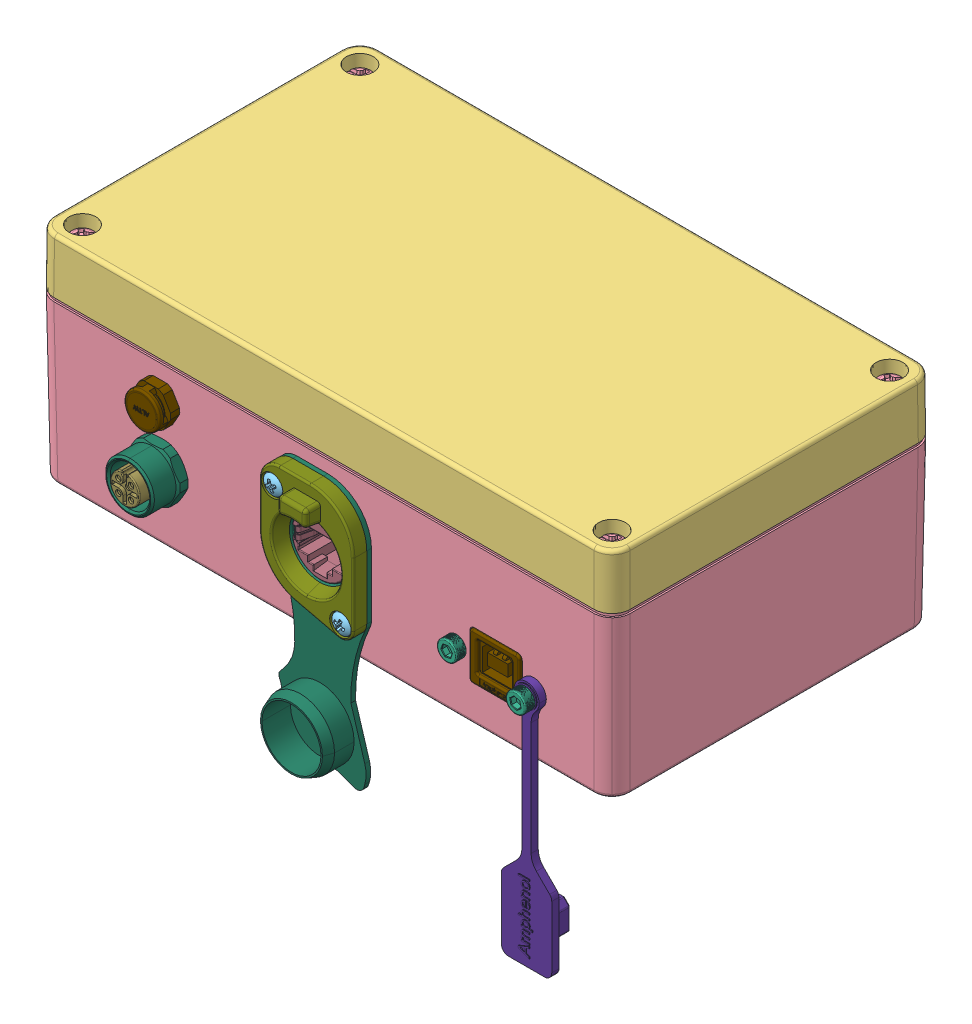
SolidWorks assembly Fleet-Monitor_V1.0, configuration Standard. Lengths in mm.
Overall size (180.3 108.03 100.3).
533 component instances, 174 part files, 48 mates.
Components (placement in the parent):
- Free-Models-1: Free-Models [Standard] x (1 0 0) z (0 1 0) size (180.29 89.97 48.51)
  - 1554J-Body-1: 1554J-Body [Standard] at (-67.276 32.873 34.5) x (1 0 0) z (0 -1 0) size (159.97 48.51 89.97)
    - 1554J.stp-1: 1554J.stp [Standard] at origin size (159.97 48.51 89.97)
      - IN100 (insert M3-0.5X5.75mm BRASS).stp-1: IN100 (insert M3-0.5X5.75mm BRASS).stp [Standard] at (128.026 -41.715 61.8734) size (4.83 5.72 4.83)
      - IN100 (insert M3-0.5X5.75mm BRASS).stp-2: IN100 (insert M3-0.5X5.75mm BRASS).stp [Standard] at (128.026 -41.715 3.8734) size (4.83 5.72 4.83)
      - IN100 (insert M3-0.5X5.75mm BRASS).stp-3: IN100 (insert M3-0.5X5.75mm BRASS).stp [Standard] at (6.526 -41.715 61.8734) size (4.83 5.72 4.83)
      - IN100 (insert M3-0.5X5.75mm BRASS).stp-4: IN100 (insert M3-0.5X5.75mm BRASS).stp [Standard] at (6.526 -41.715 3.8734) size (4.83 5.72 4.83)
      - IN-M4 (insert M4-0.7X5.75mm SS).stp-1: IN-M4 (insert M4-0.7X5.75mm SS).stp [Standard] at (-6.224 -6.35 -5.6266) size (6.35 6.35 6.35)
      - IN-M4 (insert M4-0.7X5.75mm SS).stp-2: IN-M4 (insert M4-0.7X5.75mm SS).stp [Standard] at (-6.224 -6.35 71.3734) size (6.35 6.35 6.35)
      - IN-M4 (insert M4-0.7X5.75mm SS).stp-3: IN-M4 (insert M4-0.7X5.75mm SS).stp [Standard] at (140.776 -6.35 71.3734) size (6.35 6.35 6.35)
      - IN-M4 (insert M4-0.7X5.75mm SS).stp-4: IN-M4 (insert M4-0.7X5.75mm SS).stp [Standard] at (140.776 -6.35 -5.6266) size (6.35 6.35 6.35)
      - 1554J-K GASKET.stp-1: 1554J-K GASKET.stp [Standard] at (-3.2352 3.5 71.7099) x (1 0 0) z (0 -1 0) size (157.48 87.47 1.5)
      - 1554J Box.stp-1: 1554J Box.stp [Standard] x (1 0 0) z (0 1 0) size (159.97 89.97 47.51)
  - M3 x 0.5mm Thread 6mm LONG SOCKET HEAD CAP SCREW-1: M3 x 0.5mm Thread 6mm LONG SOCKET HEAD CAP SCREW [Standard] at (0 29 -6) x (1 0 0) z (0 0 -1) size (5.5 5.5 9)
  - M3 x 0.5mm Thread 6mm LONG SOCKET HEAD CAP SCREW-2: M3 x 0.5mm Thread 6mm LONG SOCKET HEAD CAP SCREW [Standard] at (-60.75 -29 -6) x (1 0 0) z (0 0 -1) size (5.5 5.5 9)
  - M3 x 0.5mm Thread 6mm LONG SOCKET HEAD CAP SCREW-3: M3 x 0.5mm Thread 6mm LONG SOCKET HEAD CAP SCREW [Standard] at (-60.75 29 -6) x (1 0 0) z (0 0 -1) size (5.5 5.5 9)
  - M3 x 0.5mm Thread 6mm LONG SOCKET HEAD CAP SCREW-4: M3 x 0.5mm Thread 6mm LONG SOCKET HEAD CAP SCREW [Standard] at (60.75 29 -6) x (1 0 0) z (0 0 -1) size (5.5 5.5 9)
  - M3 x 0.5mm Thread 6mm LONG SOCKET HEAD CAP SCREW-5: M3 x 0.5mm Thread 6mm LONG SOCKET HEAD CAP SCREW [Standard] at (60.75 -29 -6) x (1 0 0) z (0 0 -1) size (5.5 5.5 9)
  - c-1-967402-1-d2-3d_Receptacle-1: c-1-967402-1-d2-3d_Receptacle [Standard] at (-56.0339 -0.0004 14.3035) x (0.002273 0.984808 -0.173633) z (0.999914 0 0.01309) size (36.5 35.21 44)
- C1-1: C1 [Standard] x (1 0 0) z (0 1 0) size (0.81 1.61 0.81)
  - C1-subassembly-1-1: C1-subassembly-1 [Standard] at (63.6949 12.2289 0) x (0 -1 0) z (0 0 1) size (1.61 0.81 0.81)
    - User Library-0603_Cap-1: User Library-0603_Cap [Standard] at origin size (0.41 0.81 0.81)
    - User Library-0603_Cap-1-1: User Library-0603_Cap-1 [Standard] at origin size (0.8 0.8 0.81)
    - User Library-0603_Cap-2-1: User Library-0603_Cap-2 [Standard] at origin size (0.41 0.81 0.81)
- C2-1: C2 [Standard] x (1 0 0) z (0 1 0) size (0.81 1.61 0.81)
  - C2-subassembly-1-1: C2-subassembly-1 [Standard] at (65.2501 12.2499 0) x (0 -1 0) z (0 0 1) size (1.61 0.81 0.81)
    - User Library-0603_Cap-1: User Library-0603_Cap [Standard] at origin size (0.41 0.81 0.81)
    - User Library-0603_Cap-1-1: User Library-0603_Cap-1 [Standard] at origin size (0.8 0.8 0.81)
    - User Library-0603_Cap-2-1: User Library-0603_Cap-2 [Standard] at origin size (0.41 0.81 0.81)
- C4-1: C4 [Standard] x (1 0 0) z (0 1 0) size (0.81 1.61 0.81)
  - C4-subassembly-1-1: C4-subassembly-1 [Standard] at (65.2999 -11.2999 0) x (0 1 0) z (0 0 1) size (1.61 0.81 0.81)
    - User Library-0603_Cap-1: User Library-0603_Cap [Standard] at origin size (0.41 0.81 0.81)
    - User Library-0603_Cap-1-1: User Library-0603_Cap-1 [Standard] at origin size (0.8 0.8 0.81)
    - User Library-0603_Cap-2-1: User Library-0603_Cap-2 [Standard] at origin size (0.41 0.81 0.81)
- C5-1: C5 [Standard] x (1 0 0) z (0 1 0) size (0.81 1.61 0.81)
  - C5-subassembly-1-1: C5-subassembly-1 [Standard] at (-47.4999 31.9999 0) x (0 -1 0) z (0 0 1) size (1.61 0.81 0.81)
    - User Library-0603_Cap-1: User Library-0603_Cap [Standard] at origin size (0.41 0.81 0.81)
    - User Library-0603_Cap-1-1: User Library-0603_Cap-1 [Standard] at origin size (0.8 0.8 0.81)
    - User Library-0603_Cap-2-1: User Library-0603_Cap-2 [Standard] at origin size (0.41 0.81 0.81)
- C6-1: C6 [Standard] x (1 0 0) z (0 1 0) size (0.81 1.61 0.81)
  - C6-subassembly-1-1: C6-subassembly-1 [Standard] at (-47.5001 29.0001 0) x (0 1 0) z (0 0 1) size (1.61 0.81 0.81)
    - User Library-0603_Cap-1: User Library-0603_Cap [Standard] at origin size (0.41 0.81 0.81)
    - User Library-0603_Cap-1-1: User Library-0603_Cap-1 [Standard] at origin size (0.8 0.8 0.81)
    - User Library-0603_Cap-2-1: User Library-0603_Cap-2 [Standard] at origin size (0.41 0.81 0.81)
- C7-1: C7 [Standard] x (1 0 0) z (0 1 0) size (4.5 2 1.25)
  - User Library-Ceramic_Capacitor_1808_h50mil-1: User Library-Ceramic_Capacitor_1808_h50mil [Standard] at (-22.0001 21.7499 0) x (-1 0 0) z (0 0 1) size (4.5 2 1.25)
    - CeramicBody-1: CeramicBody [Standard] at origin size (4.3 1.98 1.23)
    - Pin2-1: Pin2 [Standard] at origin size (0.77 2 1.25)
    - Pin1-1: Pin1 [Standard] at origin size (0.77 2 1.25)
- C8-1: C8 [Standard] x (1 0 0) z (0 1 0) size (1.61 0.81 0.81)
  - C8-subassembly-1-1: C8-subassembly-1 [Standard] at (-15.7501 36.9999 0) x (-1 0 0) z (0 0 1) size (1.61 0.81 0.81)
    - User Library-0603_Cap-1: User Library-0603_Cap [Standard] at origin size (0.41 0.81 0.81)
    - User Library-0603_Cap-1-1: User Library-0603_Cap-1 [Standard] at origin size (0.8 0.8 0.81)
    - User Library-0603_Cap-2-1: User Library-0603_Cap-2 [Standard] at origin size (0.41 0.81 0.81)
- C10-1: C10 [Standard] x (1 0 0) z (0 1 0) size (1.61 0.81 0.81)
  - C10-subassembly-1-1: C10-subassembly-1 [Standard] at (-30.2501 15.9999 0) x (-1 0 0) z (0 0 1) size (1.61 0.81 0.81)
    - User Library-0603_Cap-1: User Library-0603_Cap [Standard] at origin size (0.41 0.81 0.81)
    - User Library-0603_Cap-1-1: User Library-0603_Cap-1 [Standard] at origin size (0.8 0.8 0.81)
    - User Library-0603_Cap-2-1: User Library-0603_Cap-2 [Standard] at origin size (0.41 0.81 0.81)
- C11-1: C11 [Standard] x (1 0 0) z (0 1 0) size (0.81 1.61 0.81)
  - C11-subassembly-1-1: C11-subassembly-1 [Standard] at (-28.5001 31.5001 0) x (0 1 0) z (0 0 1) size (1.61 0.81 0.81)
    - User Library-0603_Cap-1: User Library-0603_Cap [Standard] at origin size (0.41 0.81 0.81)
    - User Library-0603_Cap-1-1: User Library-0603_Cap-1 [Standard] at origin size (0.8 0.8 0.81)
    - User Library-0603_Cap-2-1: User Library-0603_Cap-2 [Standard] at origin size (0.41 0.81 0.81)
- C12-1: C12 [Standard] x (1 0 0) z (0 1 0) size (0.81 1.61 0.81)
  - C12-subassembly-1-1: C12-subassembly-1 [Standard] at (-20.0001 -4.7499 0) x (0 1 0) z (0 0 1) size (1.61 0.81 0.81)
    - User Library-0603_Cap-1: User Library-0603_Cap [Standard] at origin size (0.41 0.81 0.81)
    - User Library-0603_Cap-1-1: User Library-0603_Cap-1 [Standard] at origin size (0.8 0.8 0.81)
    - User Library-0603_Cap-2-1: User Library-0603_Cap-2 [Standard] at origin size (0.41 0.81 0.81)
- C13-1: C13 [Standard] x (1 0 0) z (0 1 0) size (0.81 1.61 0.81)
  - C13-subassembly-1-1: C13-subassembly-1 [Standard] at (-18.7501 -4.7499 0) x (0 1 0) z (0 0 1) size (1.61 0.81 0.81)
    - User Library-0603_Cap-1: User Library-0603_Cap [Standard] at origin size (0.41 0.81 0.81)
    - User Library-0603_Cap-1-1: User Library-0603_Cap-1 [Standard] at origin size (0.8 0.8 0.81)
    - User Library-0603_Cap-2-1: User Library-0603_Cap-2 [Standard] at origin size (0.41 0.81 0.81)
- C14-1: C14 [Standard] x (1 0 0) z (0 1 0) size (0.81 1.61 0.81)
  - C14-subassembly-1-1: C14-subassembly-1 [Standard] at (-20.0001 -7.2499 0) x (0 1 0) z (0 0 1) size (1.61 0.81 0.81)
    - User Library-0603_Cap-1: User Library-0603_Cap [Standard] at origin size (0.41 0.81 0.81)
    - User Library-0603_Cap-1-1: User Library-0603_Cap-1 [Standard] at origin size (0.8 0.8 0.81)
    - User Library-0603_Cap-2-1: User Library-0603_Cap-2 [Standard] at origin size (0.41 0.81 0.81)
- C15-1: C15 [Standard] x (1 0 0) z (0 1 0) size (0.81 1.61 0.81)
  - C15-subassembly-1-1: C15-subassembly-1 [Standard] at (-20.0001 -2.2499 0) x (0 1 0) z (0 0 1) size (1.61 0.81 0.81)
    - User Library-0603_Cap-1: User Library-0603_Cap [Standard] at origin size (0.41 0.81 0.81)
    - User Library-0603_Cap-1-1: User Library-0603_Cap-1 [Standard] at origin size (0.8 0.8 0.81)
    - User Library-0603_Cap-2-1: User Library-0603_Cap-2 [Standard] at origin size (0.41 0.81 0.81)
- C16-1: C16 [Standard] x (1 0 0) z (0 1 0) size (1.61 0.81 0.81)
  - C16-subassembly-1-1: C16-subassembly-1 [Standard] at (-24.4999 3.0001 0) x (1 0 0) z (0 0 1) size (1.61 0.81 0.81)
    - User Library-0603_Cap-1: User Library-0603_Cap [Standard] at origin size (0.41 0.81 0.81)
    - User Library-0603_Cap-1-1: User Library-0603_Cap-1 [Standard] at origin size (0.8 0.8 0.81)
    - User Library-0603_Cap-2-1: User Library-0603_Cap-2 [Standard] at origin size (0.41 0.81 0.81)
- C21-1: C21 [Standard] x (1 0 0) z (0 1 0) size (0.81 1.61 0.81)
  - C21-subassembly-1-1: C21-subassembly-1 [Standard] at (-17.5001 -2.2499 0) x (0 1 0) z (0 0 1) size (1.61 0.81 0.81)
    - User Library-0603_Cap-1: User Library-0603_Cap [Standard] at origin size (0.41 0.81 0.81)
    - User Library-0603_Cap-1-1: User Library-0603_Cap-1 [Standard] at origin size (0.8 0.8 0.81)
    - User Library-0603_Cap-2-1: User Library-0603_Cap-2 [Standard] at origin size (0.41 0.81 0.81)
- C19-1: C19 [Standard] x (1 0 0) z (0 1 0) size (0.81 1.61 0.81)
  - C19-subassembly-1-1: C19-subassembly-1 [Standard] at (-28.7501 5.5001 0) x (0 1 0) z (0 0 1) size (1.61 0.81 0.81)
    - User Library-0603_Cap-1: User Library-0603_Cap [Standard] at origin size (0.41 0.81 0.81)
    - User Library-0603_Cap-1-1: User Library-0603_Cap-1 [Standard] at origin size (0.8 0.8 0.81)
    - User Library-0603_Cap-2-1: User Library-0603_Cap-2 [Standard] at origin size (0.41 0.81 0.81)
- C18-1: C18 [Standard] x (1 0 0) z (0 1 0) size (0.81 1.61 0.81)
  - C18-subassembly-1-1: C18-subassembly-1 [Standard] at (-23.9999 5.4999 0) x (0 -1 0) z (0 0 1) size (1.61 0.81 0.81)
    - User Library-0603_Cap-1: User Library-0603_Cap [Standard] at origin size (0.41 0.81 0.81)
    - User Library-0603_Cap-1-1: User Library-0603_Cap-1 [Standard] at origin size (0.8 0.8 0.81)
    - User Library-0603_Cap-2-1: User Library-0603_Cap-2 [Standard] at origin size (0.41 0.81 0.81)
- C20-1: C20 [Standard] x (1 0 0) z (0 1 0) size (0.81 1.61 0.81)
  - C20-subassembly-1-1: C20-subassembly-1 [Standard] at (-18.7501 -2.2499 0) x (0 1 0) z (0 0 1) size (1.61 0.81 0.81)
    - User Library-0603_Cap-1: User Library-0603_Cap [Standard] at origin size (0.41 0.81 0.81)
    - User Library-0603_Cap-1-1: User Library-0603_Cap-1 [Standard] at origin size (0.8 0.8 0.81)
    - User Library-0603_Cap-2-1: User Library-0603_Cap-2 [Standard] at origin size (0.41 0.81 0.81)
- C22-1: C22 [Standard] x (1 0 0) z (0 1 0) size (1.61 0.81 0.81)
  - C22-subassembly-1-1: C22-subassembly-1 [Standard] at (-29.2501 -16.0001 0) x (-1 0 0) z (0 0 1) size (1.61 0.81 0.81)
    - User Library-0603_Cap-1: User Library-0603_Cap [Standard] at origin size (0.41 0.81 0.81)
    - User Library-0603_Cap-1-1: User Library-0603_Cap-1 [Standard] at origin size (0.8 0.8 0.81)
    - User Library-0603_Cap-2-1: User Library-0603_Cap-2 [Standard] at origin size (0.41 0.81 0.81)
- C23-1: C23 [Standard] x (1 0 0) z (0 1 0) size (1.61 0.81 0.81)
  - C23-subassembly-1-1: C23-subassembly-1 [Standard] at (-26.4999 -20.7499 0) x (1 0 0) z (0 0 1) size (1.61 0.81 0.81)
    - User Library-0603_Cap-1: User Library-0603_Cap [Standard] at origin size (0.41 0.81 0.81)
    - User Library-0603_Cap-1-1: User Library-0603_Cap-1 [Standard] at origin size (0.8 0.8 0.81)
    - User Library-0603_Cap-2-1: User Library-0603_Cap-2 [Standard] at origin size (0.41 0.81 0.81)
- C24-1: C24 [Standard] x (1 0 0) z (0 1 0) size (1.61 0.81 0.81)
  - C24-subassembly-1-1: C24-subassembly-1 [Standard] at (-29.2501 -22.2501 0) x (-1 0 0) z (0 0 1) size (1.61 0.81 0.81)
    - User Library-0603_Cap-1: User Library-0603_Cap [Standard] at origin size (0.41 0.81 0.81)
    - User Library-0603_Cap-1-1: User Library-0603_Cap-1 [Standard] at origin size (0.8 0.8 0.81)
    - User Library-0603_Cap-2-1: User Library-0603_Cap-2 [Standard] at origin size (0.41 0.81 0.81)
- C27-1: C27 [Standard] x (1 0 0) z (0 1 0) size (4.5 2 1.25)
  - User Library-Ceramic_Capacitor_1808_h50mil-1: User Library-Ceramic_Capacitor_1808_h50mil [Standard] at (-18.9999 -27.0999 0) x (1 0 0) z (0 0 1) size (4.5 2 1.25)
    - CeramicBody-1: CeramicBody [Standard] at origin size (4.3 1.98 1.23)
    - Pin2-1: Pin2 [Standard] at origin size (0.77 2 1.25)
    - Pin1-1: Pin1 [Standard] at origin size (0.77 2 1.25)
- C25-1: C25 [Standard] x (1 0 0) z (0 1 0) size (1.61 0.81 0.81)
  - C25-subassembly-1-1: C25-subassembly-1 [Standard] at (-26.4999 -23.4999 0) x (1 0 0) z (0 0 1) size (1.61 0.81 0.81)
    - User Library-0603_Cap-1: User Library-0603_Cap [Standard] at origin size (0.41 0.81 0.81)
    - User Library-0603_Cap-1-1: User Library-0603_Cap-1 [Standard] at origin size (0.8 0.8 0.81)
    - User Library-0603_Cap-2-1: User Library-0603_Cap-2 [Standard] at origin size (0.41 0.81 0.81)
- C31-1: C31 [Standard] x (1 0 0) z (0 1 0) size (0.81 1.61 0.81)
  - C31-subassembly-1-1: C31-subassembly-1 [Standard] at (1.9999 8.5001 0) x (0 1 0) z (0 0 1) size (1.61 0.81 0.81)
    - User Library-0603_Cap-1: User Library-0603_Cap [Standard] at origin size (0.41 0.81 0.81)
    - User Library-0603_Cap-1-1: User Library-0603_Cap-1 [Standard] at origin size (0.8 0.8 0.81)
    - User Library-0603_Cap-2-1: User Library-0603_Cap-2 [Standard] at origin size (0.41 0.81 0.81)
- C28-1: C28 [Standard] x (1 0 0) z (0 1 0) size (1.25 2 0.78)
  - User Library-0805 SMD Capacitor-1: User Library-0805 SMD Capacitor [Standard] at (-4.0001 8.5001 0) x (0 1 0) z (1 0 0) size (2 0.78 1.25)
- C29-1: C29 [Standard] x (1 0 0) z (0 1 0) size (1.25 2 0.78)
  - User Library-0805 SMD Capacitor-1: User Library-0805 SMD Capacitor [Standard] at (-0.5001 8.5001 0) x (0 1 0) z (1 0 0) size (2 0.78 1.25)
- C30-1: C30 [Standard] x (1 0 0) z (0 1 0) size (1.25 2 0.78)
  - User Library-0805 SMD Capacitor-1: User Library-0805 SMD Capacitor [Standard] at (-7.5001 8.5001 0) x (0 1 0) z (1 0 0) size (2 0.78 1.25)
- C32-1: C32 [Standard] x (1 0 0) z (0 1 0) size (0.81 1.61 0.81)
  - C32-subassembly-1-1: C32-subassembly-1 [Standard] at (8.2501 -3.4601 0) x (0 -1 0) z (0 0 1) size (1.61 0.81 0.81)
    - User Library-0603_Cap-1: User Library-0603_Cap [Standard] at origin size (0.41 0.81 0.81)
    - User Library-0603_Cap-1-1: User Library-0603_Cap-1 [Standard] at origin size (0.8 0.8 0.81)
    - User Library-0603_Cap-2-1: User Library-0603_Cap-2 [Standard] at origin size (0.41 0.81 0.81)
- C33-1: C33 [Standard] x (1 0 0) z (0 1 0) size (0.81 1.61 0.81)
  - C33-subassembly-1-1: C33-subassembly-1 [Standard] at (31.2499 0.0001 0) x (0 1 0) z (0 0 1) size (1.61 0.81 0.81)
    - User Library-0603_Cap-1: User Library-0603_Cap [Standard] at origin size (0.41 0.81 0.81)
    - User Library-0603_Cap-1-1: User Library-0603_Cap-1 [Standard] at origin size (0.8 0.8 0.81)
    - User Library-0603_Cap-2-1: User Library-0603_Cap-2 [Standard] at origin size (0.41 0.81 0.81)
- C34-1: C34 [Standard] x (1 0 0) z (0 1 0) size (0.81 1.61 0.81)
  - C34-subassembly-1-1: C34-subassembly-1 [Standard] at (32.4999 0.0001 0) x (0 1 0) z (0 0 1) size (1.61 0.81 0.81)
    - User Library-0603_Cap-1: User Library-0603_Cap [Standard] at origin size (0.41 0.81 0.81)
    - User Library-0603_Cap-1-1: User Library-0603_Cap-1 [Standard] at origin size (0.8 0.8 0.81)
    - User Library-0603_Cap-2-1: User Library-0603_Cap-2 [Standard] at origin size (0.41 0.81 0.81)
- C35-1: C35 [Standard] x (1 0 0) z (0 1 0) size (0.81 1.61 0.81)
  - C35-subassembly-1-1: C35-subassembly-1 [Standard] at (29.9999 0.0001 0) x (0 1 0) z (0 0 1) size (1.61 0.81 0.81)
    - User Library-0603_Cap-1: User Library-0603_Cap [Standard] at origin size (0.41 0.81 0.81)
    - User Library-0603_Cap-1-1: User Library-0603_Cap-1 [Standard] at origin size (0.8 0.8 0.81)
    - User Library-0603_Cap-2-1: User Library-0603_Cap-2 [Standard] at origin size (0.41 0.81 0.81)
- D1-1: D1 [Standard] x (1 0 0) z (0 1 0) size (2.1 2 0.96)
  - User Library-SC70-6-1: User Library-SC70-6 [Standard] at (47.5001 -23.7501 0.5) x (0 1 0) z (1 0 0) size (2 0.96 2.1)
- D2-1: D2 [Standard] x (1 0 0) z (0 1 0) size (2.1 2 0.96)
  - User Library-SC70-6-1: User Library-SC70-6 [Standard] at (-41.3001 27.0001 0.5) x (0 -1 0) z (-1 0 0) size (2 0.96 2.1)
- D3-1: D3 [Standard] x (1 0 0) z (0 1 0) size (2 2.1 0.96)
  - User Library-SC70-6-1: User Library-SC70-6 [Standard] at (-31.7499 -10.4999 0.5) x (-1 0 0) z (0 1 0) size (2 0.96 2.1)
- D5-1: D5 [Standard] x (1 0 0) z (0 1 0) size (5.6 2.95 2.7)
  - User Library-S1G-1-1: User Library-S1G-1 [Standard] at (23.7501 -32.9999 0) x (1 0 0) z (0 0 1) size (5.6 2.95 2.7)
- D4-1: D4 [Standard] x (1 0 0) z (0 1 0) size (2.95 5.6 2.7)
  - User Library-S1G-1-1: User Library-S1G-1 [Standard] at (-44.9999 -17.5001 0) x (0 -1 0) z (0 0 1) size (5.6 2.95 2.7)
- F1-1: F1 [Standard] x (1 0 0) z (0 1 0) size (3.2 4.5 0.5)
  - F1-subassembly-1-1: F1-subassembly-1 [Standard] at (-45.0001 -24.9999 0.3) x (0 1 0) z (1 0 0) size (4.5 0.5 3.2)
    - User Library-0ZCG-0_90mm-1: User Library-0ZCG-0_90mm [Standard] at origin size (3.1 0.46 3.2)
    - User Library-0ZCG-0_90mm-1-1: User Library-0ZCG-0_90mm-1 [Standard] at origin size (0.7 0.5 3.2)
    - User Library-0ZCG-0_90mm-2-1: User Library-0ZCG-0_90mm-2 [Standard] at origin size (0.7 0.5 3.2)
    - User Library-0ZCG-0_90mm-3-1: User Library-0ZCG-0_90mm-3 [Standard] at origin size (4.5 0.17 3.2)
- F2-1: F2 [Standard] x (1 0 0) z (0 1 0) size (3.2 1.67 0.58)
  - User Library-Fuse1206-1: User Library-Fuse1206 [Standard] at (30.5 -32.9999 0) x (1 0 0) z (0 -1 0) size (3.2 0.58 1.67)
- L1-1: L1 [Standard] x (1 0 0) z (0 1 0) size (4.5 3.2 3)
  - User Library-ACT45B_GERMANY-1: User Library-ACT45B_GERMANY [Standard] at (-41.0001 31.4999 0) x (-1 0 0) z (0 0 1) size (4.5 3.2 3)
- L2-1: L2 [Standard] x (1 0 0) z (0 1 0) size (2 1.2 0.95)
  - User Library-ind_0805-1: User Library-ind_0805 [Standard] at (-18.7501 37.2499 0) x (-1 0 0) z (0 0 1) size (2 1.2 0.95)
- L4-1: L4 [Standard] x (1 0 0) z (0 1 0) size (1.2 2 0.95)
  - User Library-ind_0805-1: User Library-ind_0805 [Standard] at (4.5001 8.4999 0) x (0 -1 0) z (0 0 1) size (2 1.2 0.95)
- P1-1: P1 [Standard] x (1 0 0) z (0 1 0) size (2 2 0.9)
  - P1-subassembly-1-1: P1-subassembly-1 [Standard] at (39.2501 27.2499 0.45) x (0 -1 0) z (-1 0 0) size (2 0.9 2)
    - CLVBA-FKA-1: CLVBA-FKA [Standard] at origin size (0.61 0.4 0.56)
    - CLVBA-FKA-1-1: CLVBA-FKA-1 [Standard] at origin size (1.84 0.9 2)
    - CLVBA-FKA-2-1: CLVBA-FKA-2 [Standard] at origin size (1.58 0.46 1.58)
    - CLVBA-FKA-3-1: CLVBA-FKA-3 [Standard] at origin size (0.61 0.4 0.56)
    - CLVBA-FKA-4-1: CLVBA-FKA-4 [Standard] at origin size (0.61 0.4 0.56)
    - CLVBA-FKA-5-1: CLVBA-FKA-5 [Standard] at origin size (0.61 0.4 0.56)
- P2-1: P2 [Standard] x (1 0 0) z (0 1 0) size (2 2 0.9)
  - P2-subassembly-1-1: P2-subassembly-1 [Standard] at (39.2501 33.4999 0.45) x (0 -1 0) z (-1 0 0) size (2 0.9 2)
    - CLVBA-FKA-1: CLVBA-FKA [Standard] at origin size (0.61 0.4 0.56)
    - CLVBA-FKA-1-1: CLVBA-FKA-1 [Standard] at origin size (1.84 0.9 2)
    - CLVBA-FKA-2-1: CLVBA-FKA-2 [Standard] at origin size (1.58 0.46 1.58)
    - CLVBA-FKA-3-1: CLVBA-FKA-3 [Standard] at origin size (0.61 0.4 0.56)
    - CLVBA-FKA-4-1: CLVBA-FKA-4 [Standard] at origin size (0.61 0.4 0.56)
    - CLVBA-FKA-5-1: CLVBA-FKA-5 [Standard] at origin size (0.61 0.4 0.56)
- Q1-1: Q1 [Standard] x (1 0 0) z (0 1 0) size (2.5 2 0.7)
  - Q1-subassembly-1-1: Q1-subassembly-1 [Standard] at (-26.5 5.5 0.05) x (-1 0 0) z (0 1 0) size (2.5 0.7 2)
    - 2520 SMD Crystal Oscillator-1: 2520 SMD Crystal Oscillator [Standard] at origin size (0.65 0.25 0.65)
    - 2520 SMD Crystal Oscillator-1-1: 2520 SMD Crystal Oscillator-1 [Standard] at origin size (0.65 0.25 0.65)
    - 2520 SMD Crystal Oscillator-2-1: 2520 SMD Crystal Oscillator-2 [Standard] at origin size (0.65 0.25 0.65)
    - 2520 SMD Crystal Oscillator-3-1: 2520 SMD Crystal Oscillator-3 [Standard] at origin size (2.5 0.45 2)
    - 2520 SMD Crystal Oscillator-4-1: 2520 SMD Crystal Oscillator-4 [Standard] at origin size (0.65 0.25 0.65)
    - 2520 SMD Crystal Oscillator-5-1: 2520 SMD Crystal Oscillator-5 [Standard] at origin size (2.3 0.2 1.8)
- R1-1: R1 [Standard] x (1 0 0) z (0 1 0) size (1.6 3.2 0.52)
  - User Library-R-0603-Array-4-1-1: User Library-R-0603-Array-4-1 [Standard] at (35.4998 27.2499 0) x (0 -1 0) z (0 0 1) size (3.2 1.6 0.52)
- R2-1: R2 [Standard] x (1 0 0) z (0 1 0) size (3.2 1.6 0.52)
  - User Library-R-0603-Array-4-1-1: User Library-R-0603-Array-4-1 [Standard] at (64.4999 16.5002 0) x (-1 0 0) z (0 0 1) size (3.2 1.6 0.52)
- R3-1: R3 [Standard] x (1 0 0) z (0 1 0) size (1.6 3.2 0.52)
  - User Library-R-0603-Array-4-1-1: User Library-R-0603-Array-4-1 [Standard] at (35.4998 33.4999 0) x (0 -1 0) z (0 0 1) size (3.2 1.6 0.52)
- R4-1: R4 [Standard] x (1 0 0) z (0 1 0) size (0.82 1.6 0.45)
  - User Library-Panasonic0603-1: User Library-Panasonic0603 [Standard] at (51.2499 -16.2499 0) x (0 -1 0) z (0 0 1) size (1.6 0.82 0.45)
- R5-1: R5 [Standard] x (1 0 0) z (0 1 0) size (0.82 1.6 0.45)
  - User Library-Panasonic0603-1: User Library-Panasonic0603 [Standard] at (-45.7501 32.0001 0) x (0 -1 0) z (0 0 1) size (1.6 0.82 0.45)
- R6-1: R6 [Standard] x (1 0 0) z (0 1 0) size (0.82 1.6 0.45)
  - User Library-Panasonic0603-1: User Library-Panasonic0603 [Standard] at (-37.7501 27.0001 0) x (0 -1 0) z (0 0 1) size (1.6 0.82 0.45)
- R7-1: R7 [Standard] x (1 0 0) z (0 1 0) size (1.6 3.2 0.52)
  - User Library-R-0603-Array-4-1-1: User Library-R-0603-Array-4-1 [Standard] at (-36.5002 -0.0001 0) x (0 -1 0) z (0 0 1) size (3.2 1.6 0.52)
- R8-1: R8 [Standard] x (1 0 0) z (0 1 0) size (1.6 3.2 0.52)
  - User Library-R-0603-Array-4-1-1: User Library-R-0603-Array-4-1 [Standard] at (-36.4502 -5.6501 0) x (0 -1 0) z (0 0 1) size (3.2 1.6 0.52)
- R9-1: R9 [Standard] x (1 0 0) z (0 1 0) size (3.2 1.6 0.52)
  - User Library-R-0603-Array-4-1-1: User Library-R-0603-Array-4-1 [Standard] at (-26.9001 -28.5748 0) x (-1 0 0) z (0 0 1) size (3.2 1.6 0.52)
- R10-1: R10 [Standard] x (1 0 0) z (0 1 0) size (1.6 0.82 0.45)
  - User Library-Panasonic0603-1: User Library-Panasonic0603 [Standard] at (-26.9999 3.0001 0) x (-1 0 0) z (0 0 1) size (1.6 0.82 0.45)
- R11-1: R11 [Standard] x (1 0 0) z (0 1 0) size (1.6 0.82 0.45)
  - User Library-Panasonic0603-1: User Library-Panasonic0603 [Standard] at (-24.5001 -11.0001 0) x (1 0 0) z (0 0 1) size (1.6 0.82 0.45)
- R12-1: R12 [Standard] x (1 0 0) z (0 1 0) size (1.6 0.82 0.45)
  - User Library-Panasonic0603-1: User Library-Panasonic0603 [Standard] at (-29.2499 -17.2499 0) x (-1 0 0) z (0 0 1) size (1.6 0.82 0.45)
- R13-1: R13 [Standard] x (1 0 0) z (0 1 0) size (1.6 0.82 0.45)
  - User Library-Panasonic0603-1: User Library-Panasonic0603 [Standard] at (-29.2499 -13.4999 0) x (-1 0 0) z (0 0 1) size (1.6 0.82 0.45)
- R14-1: R14 [Standard] x (1 0 0) z (0 1 0) size (1.6 0.82 0.45)
  - User Library-Panasonic0603-1: User Library-Panasonic0603 [Standard] at (-29.2499 -14.7499 0) x (-1 0 0) z (0 0 1) size (1.6 0.82 0.45)
- R20-1: R20 [Standard] x (1 0 0) z (0 1 0) size (1.6 0.82 0.45)
  - User Library-Panasonic0603-1: User Library-Panasonic0603 [Standard] at (-29.2501 -20.7501 0) x (1 0 0) z (0 0 1) size (1.6 0.82 0.45)
- R18-1: R18 [Standard] x (1 0 0) z (0 1 0) size (0.82 1.6 0.45)
  - User Library-Panasonic0603-1: User Library-Panasonic0603 [Standard] at (-4.9999 -16.5001 0) x (0 1 0) z (0 0 1) size (1.6 0.82 0.45)
- R19-1: R19 [Standard] x (1 0 0) z (0 1 0) size (0.82 1.6 0.45)
  - User Library-Panasonic0603-1: User Library-Panasonic0603 [Standard] at (-6.2501 -18.9999 0) x (0 -1 0) z (0 0 1) size (1.6 0.82 0.45)
- R24-1: R24 [Standard] x (1 0 0) z (0 1 0) size (1.6 0.82 0.45)
  - User Library-Panasonic0603-1: User Library-Panasonic0603 [Standard] at (-29.2499 -23.4999 0) x (-1 0 0) z (0 0 1) size (1.6 0.82 0.45)
- R21-1: R21 [Standard] x (1 0 0) z (0 1 0) size (1.6 0.82 0.45)
  - User Library-Panasonic0603-1: User Library-Panasonic0603 [Standard] at (3.0001 -14.9999 0) x (-1 0 0) z (0 0 1) size (1.6 0.82 0.45)
- S1-1: S1 [Standard] x (1 0 0) z (0 1 0) size (6.4 5.1 1.5)
  - S1-subassembly-1-1: S1-subassembly-1 [Standard] at (14.2499 33.4999 0) x (-1 0 0) z (0 1 0) size (6.4 1.5 5.1)
    - User Library-LP16-1: User Library-LP16 [Standard] at origin size (4.8 0.65 4.8)
    - User Library-LP16-1-1: User Library-LP16-1 [Standard] at origin size (1.45 0.35 0.5)
    - User Library-LP16-2-1: User Library-LP16-2 [Standard] at origin size (2 0.7 2)
    - User Library-LP16-3-1: User Library-LP16-3 [Standard] at origin size (1.45 0.35 0.5)
    - User Library-LP16-4-1: User Library-LP16-4 [Standard] at origin size (5.1 1.16 5.1)
    - User Library-LP16-5-1: User Library-LP16-5 [Standard] at origin size (1.45 0.35 0.5)
    - User Library-LP16-6-1: User Library-LP16-6 [Standard] at origin size (1.45 0.35 0.5)
- T1-1: T1 [Standard] x (1 0 0) z (0 1 0) size (9.53 12.7 6.1)
  - Trans_Pulse_Electronics_Corporation_H1102NL_eec-1: Trans_Pulse_Electronics_Corporation_H1102NL_eec [Standard] at (-19 -19 -2.714) x (0 -1 0) z (0 0 1) size (12.7 9.53 6.1)
    - Trans_Pulse_Electronics_Corporation_H1102NL_eec-subassembly-1-1: Trans_Pulse_Electronics_Corporation_H1102NL_eec-subassembly-1 [Standard] at (6.35 -3.4274 8.8095) size (5.24 1.42 0)
      - Pulse-1: Pulse [Standard] at origin size (0.61 0.88 0)
      - Pulse-1-1: Pulse-1 [Standard] at origin size (0.66 0.87 0)
      - Pulse-2-1: Pulse-2 [Standard] at origin size (0.71 1.13 0)
      - Pulse-3-1: Pulse-3 [Standard] at origin size (1.47 1.42 0)
      - Pulse-4-1: Pulse-4 [Standard] at origin size (0.14 1.18 0)
      - Pulse-5-1: Pulse-5 [Standard] at origin size (0.73 0.89 0)
    - Trans_Pulse_Electronics_Corporation_H1102NL_eec-subassembly-2-1: Trans_Pulse_Electronics_Corporation_H1102NL_eec-subassembly-2 [Standard] at origin size (9.4 9.53 1.88)
      - Pins-1: Pins [Standard] at origin size (0.51 1.72 1.88)
      - Pins-1-1: Pins-1 [Standard] at origin size (0.51 1.72 1.88)
      - Pins-2-1: Pins-2 [Standard] at origin size (0.51 1.72 1.88)
      - Pins-3-1: Pins-3 [Standard] at origin size (0.51 1.72 1.88)
      - Pins-4-1: Pins-4 [Standard] at origin size (0.51 1.72 1.88)
      - Pins-5-1: Pins-5 [Standard] at origin size (0.51 1.72 1.88)
      - Pins-6-1: Pins-6 [Standard] at origin size (0.51 1.72 1.88)
      - Pins-7-1: Pins-7 [Standard] at origin size (0.51 1.72 1.88)
      - Pins-8-1: Pins-8 [Standard] at origin size (0.51 1.72 1.88)
      - Pins-9-1: Pins-9 [Standard] at origin size (0.51 1.72 1.88)
      - Pins-10-1: Pins-10 [Standard] at origin size (0.51 1.72 1.88)
      - Pins-11-1: Pins-11 [Standard] at origin size (0.51 1.72 1.88)
      - Pins-12-1: Pins-12 [Standard] at origin size (0.51 1.72 1.88)
      - Pins-13-1: Pins-13 [Standard] at origin size (0.51 1.72 1.88)
      - Pins-14-1: Pins-14 [Standard] at origin size (0.51 1.72 1.88)
      - Pins-15-1: Pins-15 [Standard] at origin size (0.51 1.72 1.88)
    - Package-1: Package [Standard] at origin size (12.7 7.11 5.97)
- U1-1: U1 [Standard] x (1 0 0) z (0 1 0) size (31 18 3.3)
  - 6084430448-1: 6084430448 [Standard] at (43.25 9 0) x (0 -1 0) z (0 0 1) size (18 31 3.3)
    - 6084430448-subassembly-1-1: 6084430448-subassembly-1 [Standard] at origin size (18 23.95 0.8)
      - Castellations-1: Castellations [Standard] at origin size (0.45 0.9 0.8)
      - Castellations-1-1: Castellations-1 [Standard] at origin size (0.9 0.45 0.8)
      - Castellations-2-1: Castellations-2 [Standard] at origin size (0.9 0.45 0.8)
      - Castellations-3-1: Castellations-3 [Standard] at origin size (0.45 0.9 0.8)
      - Castellations-4-1: Castellations-4 [Standard] at origin size (0.45 0.9 0.8)
      - Castellations-5-1: Castellations-5 [Standard] at origin size (0.45 0.9 0.8)
      - Castellations-6-1: Castellations-6 [Standard] at origin size (0.45 0.9 0.8)
      - Castellations-7-1: Castellations-7 [Standard] at origin size (0.45 0.9 0.8)
      - Castellations-8-1: Castellations-8 [Standard] at origin size (0.45 0.9 0.8)
      - Castellations-9-1: Castellations-9 [Standard] at origin size (0.45 0.9 0.8)
      - Castellations-10-1: Castellations-10 [Standard] at origin size (0.45 0.9 0.8)
      - Castellations-11-1: Castellations-11 [Standard] at origin size (0.45 0.9 0.8)
      - Castellations-12-1: Castellations-12 [Standard] at origin size (0.45 0.9 0.8)
      - Castellations-13-1: Castellations-13 [Standard] at origin size (0.45 0.9 0.8)
      - Castellations-14-1: Castellations-14 [Standard] at origin size (0.45 0.9 0.8)
      - Castellations-15-1: Castellations-15 [Standard] at origin size (0.45 0.9 0.8)
      - Castellations-16-1: Castellations-16 [Standard] at origin size (0.45 0.9 0.8)
      - Castellations-17-1: Castellations-17 [Standard] at origin size (0.45 0.9 0.8)
      - Castellations-18-1: Castellations-18 [Standard] at origin size (0.45 0.9 0.8)
      - Castellations-19-1: Castellations-19 [Standard] at origin size (0.9 0.45 0.8)
      - Castellations-20-1: Castellations-20 [Standard] at origin size (0.9 0.45 0.8)
      - Castellations-21-1: Castellations-21 [Standard] at origin size (0.9 0.45 0.8)
      - Castellations-22-1: Castellations-22 [Standard] at origin size (0.9 0.45 0.8)
      - Castellations-23-1: Castellations-23 [Standard] at origin size (0.9 0.45 0.8)
      - Castellations-24-1: Castellations-24 [Standard] at origin size (0.45 0.9 0.8)
      - Castellations-25-1: Castellations-25 [Standard] at origin size (0.45 0.9 0.8)
      - Castellations-26-1: Castellations-26 [Standard] at origin size (0.45 0.9 0.8)
      - Castellations-27-1: Castellations-27 [Standard] at origin size (0.45 0.9 0.8)
      - Castellations-28-1: Castellations-28 [Standard] at origin size (0.45 0.9 0.8)
      - Castellations-29-1: Castellations-29 [Standard] at origin size (0.45 0.9 0.8)
      - Castellations-30-1: Castellations-30 [Standard] at origin size (0.45 0.9 0.8)
      - Castellations-31-1: Castellations-31 [Standard] at origin size (0.45 0.9 0.8)
      - Castellations-32-1: Castellations-32 [Standard] at origin size (0.45 0.9 0.8)
      - Castellations-33-1: Castellations-33 [Standard] at origin size (0.45 0.9 0.8)
      - Castellations-34-1: Castellations-34 [Standard] at origin size (0.45 0.9 0.8)
      - Castellations-35-1: Castellations-35 [Standard] at origin size (0.45 0.9 0.8)
      - Castellations-36-1: Castellations-36 [Standard] at origin size (0.45 0.9 0.8)
      - Castellations-37-1: Castellations-37 [Standard] at origin size (0.45 0.9 0.8)
      - Castellations-38-1: Castellations-38 [Standard] at origin size (0.45 0.9 0.8)
      - Castellations-39-1: Castellations-39 [Standard] at origin size (0.9 0.45 0.8)
      - Castellations-40-1: Castellations-40 [Standard] at origin size (0.9 0.45 0.8)
      - Castellations-41-1: Castellations-41 [Standard] at origin size (0.9 0.45 0.8)
    - Can-1: Can [Standard] at origin size (15.84 23.1 2.5)
    - UFL Connector-1: UFL Connector [Standard] at origin size (3.1 3 1.25)
    - Trace Antenna-1: Trace Antenna [Standard] at origin size (15 5.5 0.1)
    - PCB-1: PCB [Standard] at origin size (18 31 0.8)
